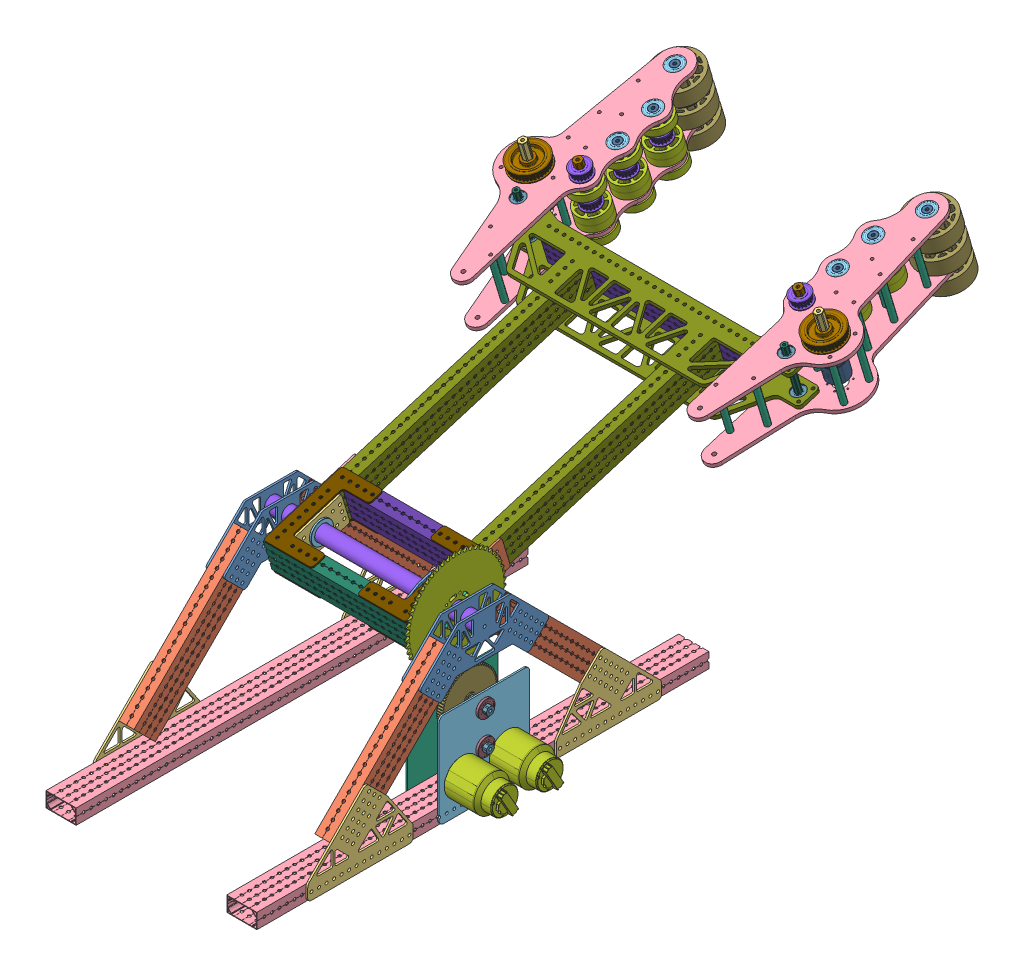
SolidWorks assembly Claw Assembly, configuration Default. Lengths in mm.
Overall size (590.37 576.41 1182.94).
222 component instances, 53 part files, 14 mates.
Components (placement in the parent):
- Side Assem 1-1: Side Assem 1 [Default] at (355.6 100.2071 0) size (53.97 279.4 762)
  - Top Gussest-1: Top Gussest [Default] at (-355.6 -95.25 -762) x (-1 0 0) z (0 0 -1) size (3.17 99.23 215.52)
  - Top Gussest-2: Top Gussest [Default] at (-330.2 -95.25 0) size (3.17 99.23 215.52)
  - 10.75in-1: 10.75in [Default] at (-342.9 31.4309 -149.9019) x (-1 0 0) z (0 -0.707107 0.707107) size (25.4 50.8 273.05)
  - 10.75in-2: 10.75in [Default] at (-342.9 31.4309 -612.0981) x (-1 0 0) z (0 -0.707107 -0.707107) size (25.4 50.8 273.05)
  - Bottom Gussest-1: Bottom Gussest [Default] at (-358.775 -95.25 0) size (3.17 121.55 177.8)
  - Bottom Gussest-2: Bottom Gussest [Default] at (-355.6 -95.25 -762) x (-1 0 0) z (0 0 -1) size (3.17 121.55 177.8)
  - 30in-1: 30in [Default] at (-330.2 -12.7 -12.7) x (0 -1 0) z (0 0 1) size (25.4 50.8 762)
- Side Assem 2-1: Side Assem 2 [Default] at (645.1703 93.5733 0) size (53.97 279.4 762)
  - Top Gussest-1: Top Gussest [Default] at (-289.5703 -88.6163 0) size (3.17 99.23 215.52)
  - Top Gussest-2: Top Gussest [Default] at (-314.9703 -88.6163 -762) x (-1 0 0) z (0 0 -1) size (3.17 99.23 215.52)
  - 10.75in-1: 10.75in [Default] at (-302.2703 38.0646 -612.0981) x (1 0 0) z (0 -0.707107 -0.707107) size (25.4 50.8 273.05)
  - 10.75in-2: 10.75in [Default] at (-302.2703 38.0646 -149.9019) x (1 0 0) z (0 -0.707107 0.707107) size (25.4 50.8 273.05)
  - Bottom Gussest-1: Bottom Gussest [Default] at (-286.3953 -88.6163 -762) x (-1 0 0) z (0 0 -1) size (3.17 121.55 177.8)
  - Bottom Gussest-2: Bottom Gussest [Default] at (-289.5703 -88.6163 0) size (3.17 121.55 177.8)
  - 30in-1: 30in [Default] at (-314.9703 -6.0663 -12.7) x (0 -1 0) z (0 0 1) size (25.4 50.8 762)
- Gearbox-1: Gearbox [Default] at (404.2822 133.0727 -812.0785) x (0 0 1) z (-1 0 0) size (152.4 182.49 147.05) (flexible)
  - Gearbox Plate-1: Gearbox Plate [Default] at (431.0785 -32.8657 46.1422) size (152.4 158.75 2.54)
  - Gearbox Plate 2-1: Gearbox Plate 2 [Default] at (431.0785 -32.8657 102.0222) x (-1 0 0) z (0 0 -1) size (152.4 158.75 2.54)
  - Falcon500_217-6515-1: Falcon500_217-6515 [Default] at (392.9785 -4.1633 19.9422) x (-1 0 0) z (0 0 1) size (60 60 115.81)
  - Falcon500_217-6515-2: Falcon500_217-6515 [Default] at (469.1785 -4.1633 19.9422) x (-1 0 0) z (0 0 1) size (60 60 115.81)
  - 12T Steel Spur Gear (20 DP, Falcon Motor) (217-6919).step-1: 12T Steel Spur Gear (20 DP, Falcon Motor) (217-6919).step [Default] at (392.9785 -4.1633 59.6672) x (-0.630647 0.77607 0) z (0 0 1) size (17.78 17.78 19.05)
  - 12T Steel Spur Gear (20 DP, Falcon Motor) (217-6919).step-2: 12T Steel Spur Gear (20 DP, Falcon Motor) (217-6919).step [Default] at (469.1785 -4.1633 59.6672) x (0.9345 -0.355964 0) z (0 0 1) size (17.78 17.78 19.05)
  - 15t steel hub sprocket hex boreWCP-0762-1: 15t steel hub sprocket hex boreWCP-0762 [Default] at (431.0785 76.9893 94.7959) x (-0.863195 -0.50487 0) z (0 0 -1) size (50.3 50.51 10.68)
  - 16T-1: 16T [Default] at (431.0785 21.1093 75.5935) x (-0.322756 0.946482 0) z (0 0 1) size (22.59 22.59 12.65)
  - 60T-1: 60T [Default] at (431.0785 21.1093 58.1818) x (0.322756 -0.946482 0) z (0 0 1) size (78.68 78.68 12.65)
  - 72T-2: 72T [Default] at (431.0785 76.9893 75.3268) x (-0.005633 0.999984 0) z (0 0 1) size (93.93 93.93 12.65)
  - Bearing-1: Bearing [Default] at (431.0785 21.1093 46.3009) x (0.706738 0.707475 0) z (0 0 1) size (31.12 31.12 7.94)
  - Bearing-3: Bearing [Default] at (431.0785 76.9893 101.8634) x (-0.628259 -0.778004 0) z (0 0 -1) size (31.12 31.12 7.94)
  - Bearing-4: Bearing [Default] at (431.0785 21.1093 101.8634) x (1 0 0) z (0 0 -1) size (31.12 31.12 7.94)
  - Bearing-5: Bearing [Default] at (431.0785 76.9893 46.3009) x (0.923728 0.383049 0) z (0 0 1) size (31.12 31.12 7.94)
  - Hex Stock-1: Hex Stock [Default] at (431.0785 21.1093 493.1822) x (0.752756 -0.658299 0) z (0 0 1) size (13.74 12.75 76.2)
  - Hex Stock-2: Hex Stock [Default] at (431.0785 76.9893 493.1822) x (-0.999984 -0.005633 0) z (0 0 1) size (13.74 12.75 76.2)
- Arm-1: Arm [Default] at (53.34 286.0719 -327.6042) x (1 0 0) z (0 -0.29021 0.956963) size (355.6 231.1 598.11) (flexible)
  - arm_tube_cross_back 9.5in-1: arm_tube_cross_back 9.5in [Default] at (228.6 25.4 -12.7) x (0 0 -1) z (1 0 0) size (25.4 50.8 241.3)
  - arm_tube 20.5in-1: arm_tube 20.5in [Default] at (228.6 25.4 -533.4) x (1 0 0) z (0 0 -1) size (25.4 50.8 520.7)
  - arm_tube 20.5in-2: arm_tube 20.5in [Default] at (12.7 25.4 -533.4) x (1 0 0) z (0 0 -1) size (25.4 50.8 520.7)
  - arm_tube_cross_front 7.5in-1: arm_tube_cross_front 7.5in [Default] at (38.1 25.4 -127) x (0 0 1) z (-1 0 0) size (25.4 50.8 190.5)
  - arm_body_bracket-1: arm_body_bracket [Default] at (-57.15 50.8 -457.2) x (0 0 1) z (0 1 0) size (139.7 82.55 2.54)
  - arm_body_bracket-2: arm_body_bracket [Default] at (298.45 53.34 -457.2) x (0 0 1) z (0 -1 0) size (139.7 82.55 2.54)
  - arm_pivot_mount_short-1: arm_pivot_mount_short [Default] at (212.725 25.4 -533.4) x (0 0 -1) z (1 0 0) size (82.55 63.5 3.17)
  - arm_pivot_mount-1: arm_pivot_mount [Default] at (241.3 25.4 -533.4) x (0 0 -1) z (1 0 0) size (139.7 63.5 3.17)
  - arm_pivot_short-1: arm_pivot_short [Default] at (25.4 25.4 -533.4) x (0 0 -1) z (1 0 0) size (82.55 50.8 3.17)
  - arm_pivot-1: arm_pivot [Default] at (-3.175 25.4 -533.4) x (0 0 -1) z (1 0 0) size (139.7 50.8 3.17)
  - 6338K436_Oil-Embedded Flanged Sleeve Bearing-2: 6338K436_Oil-Embedded Flanged Sleeve Bearing [6338K436] at (3.175 25.4 -63.5) x (0 -0.410084 -0.912048) z (-1 0 0) size (38.1 38.1 19.05)
  - 6338K436_Oil-Embedded Flanged Sleeve Bearing-3: 6338K436_Oil-Embedded Flanged Sleeve Bearing [6338K436] at (22.225 25.4 -63.5) x (0 -0.686347 0.727274) z (1 0 0) size (38.1 38.1 19.05)
  - 6338K436_Oil-Embedded Flanged Sleeve Bearing-4: 6338K436_Oil-Embedded Flanged Sleeve Bearing [6338K436] at (219.075 25.4 -63.5) x (0 -0.517801 -0.855501) z (-1 0 0) size (38.1 38.1 19.05)
  - 6338K436_Oil-Embedded Flanged Sleeve Bearing-5: 6338K436_Oil-Embedded Flanged Sleeve Bearing [6338K436] at (238.125 25.4 -63.5) x (0 -0.686347 0.727274) z (1 0 0) size (38.1 38.1 19.05)
  - arm_body_bracket-3: arm_body_bracket [Default] at (-57.15 -2.54 -457.2) x (0 0 1) z (0 1 0) size (139.7 82.55 2.54)
  - arm_body_bracket-4: arm_body_bracket [Default] at (298.45 0 -457.2) x (0 0 1) z (0 -1 0) size (139.7 82.55 2.54)
  - 3_8in spacer WCP-0309-1: 3_8in spacer WCP-0309 [Default] at (249.2375 46.0222 -75.4063) x (1 0 0) z (0 0.686347 -0.727274) size (9.53 9.5 9.5)
  - 54t #35 chain plate sprocket 217_2645-1: 54t #35 chain plate sprocket 217_2645 [Default] at (256.1463 25.4 -63.5) x (0 0.5 -0.866025) z (1 0 0) size (169.04 169.25 4.3)
  - 3_8in spacer WCP-0309-2: 3_8in spacer WCP-0309 [Default] at (249.2375 4.7778 -51.5938) x (1 0 0) z (0 0.686347 -0.727274) size (9.53 9.5 9.5)
  - 3_8in spacer WCP-0309-3: 3_8in spacer WCP-0309 [Default] at (249.2375 4.7778 -75.4063) x (1 0 0) z (0 0.686347 -0.727274) size (9.53 9.5 9.5)
  - 3_8in spacer WCP-0309-4: 3_8in spacer WCP-0309 [Default] at (249.2375 25.4 -39.6875) x (1 0 0) z (0 0.686347 -0.727274) size (9.53 9.5 9.5)
  - 3_8in spacer WCP-0309-5: 3_8in spacer WCP-0309 [Default] at (249.2375 46.0222 -51.5938) x (1 0 0) z (0 0.686347 -0.727274) size (9.53 9.5 9.5)
  - 3_8in spacer WCP-0309-6: 3_8in spacer WCP-0309 [Default] at (249.2375 25.4 -87.3125) x (1 0 0) z (0 0.686347 -0.727274) size (9.53 9.5 9.5)
  - tubemount-1: tubemount [Default] at (-53.34 25.4 -63.5) x (0 0.686347 -0.727274) z (-1 0 0) size (25.4 25.4 355.6)
- Roller Claw-1: Roller Claw [Default] at (-95.9547 241.4869 -1673.2272) x (1 0 0) z (0 -0.29021 0.956963) size (590.37 159.05 455.23)
  - Right Roller Claw-1: Right Roller Claw [Default] at (339.7553 150.3563 318.0728) size (145.49 159.05 454.48)
    - 36T_HTD_5mmP_9mmW_flanged_500_hex_217-3231-1: 36T_HTD_5mmP_9mmW_flanged_500_hex_217-3231 [Default] at (179.6545 359.9234 345.8295) x (-0.337159 0 -0.941448) z (0 -1 0) size (60 60 14.5)
    - ultraplanetary-1: ultraplanetary [Default] at (198.2743 320.0734 349.6112) x (-0.199034 0 0.979992) z (0 -1 0) size (63.81 63.81 121.86)
      - REV-21-1651-1: REV-21-1651 [Default] at (0 19 -11.5) x (0 0 1) z (-0.999972 -0.007497 0) size (56.01 42.91 43.01)
      - REV-41-1601-1: REV-41-1601 [Default] at (0 19 -10) x (-0.5 -0.866025 0) z (0 0 1) size (43.62 38.42 17.88)
      - REV-41-1604-1: REV-41-1604 [Default] at (0 19 -26.25) x (-0.5 0.866025 0) z (0 0 1) size (54.69 56.73 18.25)
        - REV-41-1604.STEP-1: REV-41-1604.STEP [Default] at origin size (54.69 56.73 18.25)
          - REV-41-1604-2.STEP-1: REV-41-1604-2.STEP [Default] at origin size (43.57 38 6.25)
          - REV-41-1604-1.STEP-1: REV-41-1604-1.STEP [Default] at (0 0 7) x (0.5 0.866025 0) z (0 0 -1) size (43.57 38 7.03)
          - 6704ZZ.STEP-1: 6704ZZ.STEP [Default] at (0 0 7.75) x (0.995 -0.099871 0) z (0 0 1) size (27 27 4)
          - 6704ZZ.STEP-2: 6704ZZ.STEP [Default] at (0 0 3) x (0.993119 0.117109 0) z (0 0 1) size (27 27 4)
          - REV-40-1606_Through Hole.STEP-1: REV-40-1606_Through Hole.STEP [Default] at (0 0 10.95) x (-0.517794 -0.855505 0) z (0 0 -1) size (22 22 16.95)
          - REV-41-1604-4.STEP-1: REV-41-1604-4.STEP [Default] at (0 0 9.7) x (0.517794 0.855505 0) z (0 0 1) size (22 22 1.25)
          - REV-41-1604-3.STEP-1: REV-41-1604-3.STEP [Default] at (0 0 5) size (27.02 27 1.12)
          - socket head cap screw_am_B18.3.1M - 2 x 0.4 x 4 Hex SHCS -- 4NHX.STEP-1: socket head cap screw_am_B18.3.1M - 2 x 0.4 x 4 Hex SHCS -- 4NHX.STEP [Default] at (-11.8435 -10.7579 11.2) x (0 0 -1) z (-0.492915 -0.870077 0) size (6 3.8 3.8)
          - socket head cap screw_am_B18.3.1M - 2 x 0.4 x 4 Hex SHCS -- 4NHX.STEP-2: socket head cap screw_am_B18.3.1M - 2 x 0.4 x 4 Hex SHCS -- 4NHX.STEP [Default] at (-3.3948 15.6357 11.2) x (0 0 -1) z (-0.934724 -0.355374 0) size (6 3.8 3.8)
          - socket head cap screw_am_B18.3.1M - 2 x 0.4 x 4 Hex SHCS -- 4NHX.STEP-3: socket head cap screw_am_B18.3.1M - 2 x 0.4 x 4 Hex SHCS -- 4NHX.STEP [Default] at (15.2383 -4.8778 11.2) x (0 0 -1) z (0.970727 -0.240185 0) size (6 3.8 3.8)
          - 91294A003_BLACK ALLOY STEEL FLAT-HEAD SOCKET CAP SCREW_91294A003.STEP-1: 91294A003_BLACK ALLOY STEEL FLAT-HEAD SOCKET CAP SCREW_91294A003.STEP [Default] at (6.5084 3.5803 10.95) size (4 4 5)
          - 91294A003_BLACK ALLOY STEEL FLAT-HEAD SOCKET CAP SCREW_91294A003.STEP-2: 91294A003_BLACK ALLOY STEEL FLAT-HEAD SOCKET CAP SCREW_91294A003.STEP [Default] at (-0.1535 -7.4266 10.95) size (4 4 5)
          - 91294A003_BLACK ALLOY STEEL FLAT-HEAD SOCKET CAP SCREW_91294A003.STEP-3: 91294A003_BLACK ALLOY STEEL FLAT-HEAD SOCKET CAP SCREW_91294A003.STEP [Default] at (-6.3549 3.8463 10.95) size (4 4 5)
      - REV-41-1607-1: REV-41-1607 [Default] at (0 19 0) x (-1 0 0) z (0 -1 0) size (43.57 5 38.01)
      - REV-41-1620-1: REV-41-1620 [Default] at (0 19 -32.25) x (0.876175 0.481992 0) z (0 0 1) size (22 22 46.85)
    - Claw Plates-2: Claw Plates [Default] at (-69.8106 346.3234 416.9495) size (132.77 6.35 429.09)
    - thunderhex_flanged_217-4006-10: thunderhex_flanged_217-4006 [Default] at (115.7867 348.7046 321.0569) x (0.592492 0 0.805576) z (0 -1 0) size (31.12 31.12 7.94)
    - thunderhex_flanged_217-4006-11: thunderhex_flanged_217-4006 [Default] at (115.7867 348.7046 258.5475) x (-0.906539 0 -0.422123) z (0 -1 0) size (31.12 31.12 7.94)
    - thunderhex_flanged_217-4006-12: thunderhex_flanged_217-4006 [Default] at (115.7867 348.7046 196.0381) x (-0.994435 0 -0.105355) z (0 -1 0) size (31.12 31.12 7.94)
    - thunderhex_flanged_217-4006-13: thunderhex_flanged_217-4006 [Default] at (142.9222 348.7046 129.5022) x (0.097157 0 0.995269) z (0 -1 0) size (31.12 31.12 7.94)
    - Claw Plates-1: Claw Plates [Default] at (-69.8106 263.7734 416.9495) size (132.77 6.35 429.09)
    - thunderhex_flanged_217-4006-1: thunderhex_flanged_217-4006 [Default] at (115.7867 267.7421 321.0569) x (0.900767 0 -0.434303) z (0 1 0) size (31.12 31.12 7.94)
    - thunderhex_flanged_217-4006-3: thunderhex_flanged_217-4006 [Default] at (115.7867 267.7421 258.5475) x (-0.989804 0 -0.142438) z (0 1 0) size (31.12 31.12 7.94)
    - thunderhex_flanged_217-4006-4: thunderhex_flanged_217-4006 [Default] at (115.7867 267.7421 196.0381) x (-0.890133 0 -0.4557) z (0 1 0) size (31.12 31.12 7.94)
    - thunderhex_flanged_217-4006-5: thunderhex_flanged_217-4006 [Default] at (142.9222 267.7421 129.5022) x (-0.890133 0 -0.4557) z (0 1 0) size (31.12 31.12 7.94)
    - 3_000_L_10_thru_WCP-0209-1: 3_000_L_10_thru_WCP-0209 [Default] at (120.1277 308.2234 477.6333) x (0 1 0) z (-0.241352 0 0.970438) size (76.2 9.5 9.5)
    - 3_000_L_10_thru_WCP-0209-2: 3_000_L_10_thru_WCP-0209 [Default] at (151.8777 308.2234 444.6133) x (0 1 0) z (-0.241352 0 0.970438) size (76.2 9.5 9.5)
    - 3_000_L_10_thru_WCP-0209-3: 3_000_L_10_thru_WCP-0209 [Default] at (141.5239 308.2234 345.4022) x (0 1 0) z (-0.241352 0 0.970438) size (76.2 9.5 9.5)
    - 3_000_L_10_thru_WCP-0209-4: 3_000_L_10_thru_WCP-0209 [Default] at (207.4135 308.2234 368.0545) x (0 1 0) z (-0.241352 0 0.970438) size (76.2 9.5 9.5)
    - 3_000_L_10_thru_WCP-0209-5: 3_000_L_10_thru_WCP-0209 [Default] at (207.4135 308.2234 323.6045) x (0 -1 0) z (-0.328723 0 0.944426) size (76.2 9.5 9.5)
    - 3_000_L_10_thru_WCP-0209-6: 3_000_L_10_thru_WCP-0209 [Default] at (170.8852 308.2234 287.9041) x (0 1 0) z (-0.241352 0 0.970438) size (76.2 9.5 9.5)
    - 3_000_L_10_thru_WCP-0209-7: 3_000_L_10_thru_WCP-0209 [Default] at (141.5239 308.2234 288.2522) x (0 1 0) z (-0.241352 0 0.970438) size (76.2 9.5 9.5)
    - 3_000_L_10_thru_WCP-0209-8: 3_000_L_10_thru_WCP-0209 [Default] at (166.9239 308.2234 237.2588) x (0 1 0) z (-0.241352 0 0.970438) size (76.2 9.5 9.5)
    - 3_000_L_10_thru_WCP-0209-9: 3_000_L_10_thru_WCP-0209 [Default] at (141.5239 308.2234 224.7522) x (0 1 0) z (-0.241352 0 0.970438) size (76.2 9.5 9.5)
    - 3_000_L_10_thru_WCP-0209-10: 3_000_L_10_thru_WCP-0209 [Default] at (161.9722 308.2234 173.9522) x (0 1 0) z (-0.241352 0 0.970438) size (76.2 9.5 9.5)
    - 2_OD_30A_Straight_Flex_Wheel_217-6353-1: 2_OD_30A_Straight_Flex_Wheel_217-6353 [Default] at (115.7867 293.7234 321.0569) x (-0.99292 0 0.118786) z (0.118786 0 0.99292) size (50.8 12.7 50.8)
    - 18T_HTD_5mmP_9mmW_flanged_500_hex_217-3225-2: 18T_HTD_5mmP_9mmW_flanged_500_hex_217-3225 [Default] at (115.7867 307.3234 321.0569) x (-0.800501 0 0.599331) z (0 -1 0) size (32 32 14.5)
    - 18T_HTD_5mmP_9mmW_flanged_500_hex_217-3225-1: 18T_HTD_5mmP_9mmW_flanged_500_hex_217-3225 [Default] at (115.7867 321.8234 321.0569) x (-0.800501 0 0.599331) z (0 1 0) size (32 32 14.5)
    - 2_OD_30A_Straight_Flex_Wheel_217-6353-3: 2_OD_30A_Straight_Flex_Wheel_217-6353 [Default] at (115.7867 335.4234 321.0569) x (-0.99292 0 0.118786) z (0.118786 0 0.99292) size (50.8 12.7 50.8)
    - 2_OD_30A_Straight_Flex_Wheel_217-6353-2: 2_OD_30A_Straight_Flex_Wheel_217-6353 [Default] at (115.7867 281.0234 321.0569) x (-0.99292 0 0.118786) z (0.118786 0 0.99292) size (50.8 12.7 50.8)
    - 2_OD_30A_Straight_Flex_Wheel_217-6353-13: 2_OD_30A_Straight_Flex_Wheel_217-6353 [Default] at (115.7867 257.4234 321.0569) x (-0.99292 0 0.118786) z (0.118786 0 0.99292) size (50.8 12.7 50.8)
    - 1_2thunderhex_5.5in-1: 1_2thunderhex_5.5in [Default] at (115.7867 695.5734 321.0569) x (-0.919287 0 -0.393589) z (0 -1 0) size (13.74 12.75 139.7)
    - 18T_HTD_5mmP_9mmW_flanged_500_hex_217-3225-9: 18T_HTD_5mmP_9mmW_flanged_500_hex_217-3225 [Default] at (115.7867 359.9234 321.0569) x (-0.800501 0 0.599331) z (0 -1 0) size (32 32 14.5)
    - 2_OD_30A_Straight_Flex_Wheel_217-6353-7: 2_OD_30A_Straight_Flex_Wheel_217-6353 [Default] at (115.7867 293.7234 258.5475) x (-0.956763 0 0.290869) z (0.290869 0 0.956763) size (50.8 12.7 50.8)
    - 18T_HTD_5mmP_9mmW_flanged_500_hex_217-3225-5: 18T_HTD_5mmP_9mmW_flanged_500_hex_217-3225 [Default] at (115.7867 307.3234 258.5475) x (-0.683146 0 0.730282) z (0 -1 0) size (32 32 14.5)
    - 18T_HTD_5mmP_9mmW_flanged_500_hex_217-3225-6: 18T_HTD_5mmP_9mmW_flanged_500_hex_217-3225 [Default] at (115.7867 321.8234 258.5475) x (-0.683146 0 0.730282) z (0 1 0) size (32 32 14.5)
    - 2_OD_30A_Straight_Flex_Wheel_217-6353-8: 2_OD_30A_Straight_Flex_Wheel_217-6353 [Default] at (115.7867 335.4234 258.5475) x (-0.956763 0 0.290869) z (0.290869 0 0.956763) size (50.8 12.7 50.8)
    - 2_OD_30A_Straight_Flex_Wheel_217-6353-9: 2_OD_30A_Straight_Flex_Wheel_217-6353 [Default] at (115.7867 281.0234 258.5475) x (-0.956763 0 0.290869) z (0.290869 0 0.956763) size (50.8 12.7 50.8)
    - 1_2thunderhex_4.5in-2: 1_2thunderhex_4.5in [Default] at (115.7867 695.5734 258.5475) x (0.683146 0 -0.730282) z (0 -1 0) size (13.74 12.75 114.3)
    - 2_OD_30A_Straight_Flex_Wheel_217-6353-14: 2_OD_30A_Straight_Flex_Wheel_217-6353 [Default] at (115.7867 257.4234 258.5475) x (-0.730282 0 -0.683146) z (-0.683146 0 0.730282) size (50.8 12.7 50.8)
    - 2_OD_30A_Straight_Flex_Wheel_217-6353-10: 2_OD_30A_Straight_Flex_Wheel_217-6353 [Default] at (115.7867 293.7234 196.0381) x (0.94551 0 -0.325593) z (-0.325593 0 -0.94551) size (50.8 12.7 50.8)
    - 18T_HTD_5mmP_9mmW_flanged_500_hex_217-3225-7: 18T_HTD_5mmP_9mmW_flanged_500_hex_217-3225 [Default] at (115.7867 307.3234 196.0381) x (0.656039 0 -0.754727) z (0 -1 0) size (32 32 14.5)
    - 18T_HTD_5mmP_9mmW_flanged_500_hex_217-3225-8: 18T_HTD_5mmP_9mmW_flanged_500_hex_217-3225 [Default] at (115.7867 321.8234 196.0381) x (0.656039 0 -0.754727) z (0 1 0) size (32 32 14.5)
    - 2_OD_30A_Straight_Flex_Wheel_217-6353-11: 2_OD_30A_Straight_Flex_Wheel_217-6353 [Default] at (115.7867 335.4234 196.0381) x (0.94551 0 -0.325593) z (-0.325593 0 -0.94551) size (50.8 12.7 50.8)
    - 2_OD_30A_Straight_Flex_Wheel_217-6353-12: 2_OD_30A_Straight_Flex_Wheel_217-6353 [Default] at (115.7867 281.0234 196.0381) x (0.94551 0 -0.325593) z (-0.325593 0 -0.94551) size (50.8 12.7 50.8)
    - 1_2thunderhex_4.5in-3: 1_2thunderhex_4.5in [Default] at (115.7867 695.5734 196.0381) x (0.656039 0 -0.754727) z (0 -1 0) size (13.74 12.75 114.3)
    - 2_OD_30A_Straight_Flex_Wheel_217-6353-15: 2_OD_30A_Straight_Flex_Wheel_217-6353 [Default] at (115.7867 257.4234 196.0381) x (-0.190783 0 0.981632) z (0.981632 0 0.190783) size (50.8 12.7 50.8)
    - wide_roller_wheel-1: wide_roller_wheel [Default] at (123.4101 254.2514 114.098) x (-0.521403 0 0.853311) z (-0.853311 0 -0.521403) size (76.2 25.4 76.2)
      - wide_wheel_mount-1: wide_wheel_mount [Default] at (2.9708 21.322 -24.6817) size (28.57 25.4 28.57)
      - 3_OD_30A_Straight_Flex_Wheel-1: 3_OD_30A_Straight_Flex_Wheel [Default] at (2.9708 34.022 -24.6817) size (76.2 25.4 76.2)
    - wide_roller_wheel-2: wide_roller_wheel [Default] at (123.4101 294.1514 114.098) x (-0.521403 0 0.853311) z (-0.853311 0 -0.521403) size (76.2 25.4 76.2)
      - wide_wheel_mount-1: wide_wheel_mount [Default] at (2.9708 21.322 -24.6817) size (28.57 25.4 28.57)
      - 3_OD_30A_Straight_Flex_Wheel-1: 3_OD_30A_Straight_Flex_Wheel [Default] at (2.9708 34.022 -24.6817) size (76.2 25.4 76.2)
    - 30T_HTD_5mmP_9mmW_flanged_500_hex_217-3229-2: 30T_HTD_5mmP_9mmW_flanged_500_hex_217-3229 [Default] at (142.9222 308.2234 129.5022) x (0.521403 0 -0.853311) z (0 1 0) size (51 51 14.5)
    - 1_2thunderhex_4.5in-4: 1_2thunderhex_4.5in [Default] at (142.9222 695.5734 129.5022) x (-0.99969 0 -0.024892) z (0 -1 0) size (13.74 12.75 114.3)
    - wide_roller_wheel-3: wide_roller_wheel [Default] at (162.4344 217.0514 144.9063) x (0.521403 0 -0.853311) z (0.853311 0 0.521403) size (76.2 25.4 76.2)
      - wide_wheel_mount-1: wide_wheel_mount [Default] at (2.9708 21.322 -24.6817) size (28.57 25.4 28.57)
      - 3_OD_30A_Straight_Flex_Wheel-1: 3_OD_30A_Straight_Flex_Wheel [Default] at (2.9708 34.022 -24.6817) size (76.2 25.4 76.2)
    - thunderhex_375_flanged_217-5829-1: thunderhex_375_flanged_217-5829 [Default] at (156.2494 344.7359 391.5495) x (0 1 0) z (-0.397184 0 0.917739) size (7.11 24.61 24.61)
    - thunderhex_375_flanged_217-5829-2: thunderhex_375_flanged_217-5829 [Default] at (156.2494 271.7109 391.5495) x (0 -1 0) z (0 0 1) size (7.11 24.61 24.61)
    - 3_8thunderhex_4.5in-1: 3_8thunderhex_4.5in [Default] at (156.2494 -91.8266 391.5495) x (0.142102 0 -0.989852) z (0 -1 0) size (10.24 9.53 114.3)
    - thunderhex_375_flanged_217-5829-3: thunderhex_375_flanged_217-5829 [Default] at (156.2494 274.8859 391.5495) x (0 1 0) z (0.329672 0 -0.944096) size (7.11 24.61 24.61)
    - thunderhex_375_flanged_217-5829-4: thunderhex_375_flanged_217-5829 [Default] at (156.2494 341.5609 391.5495) x (0 -1 0) z (0.640533 0 0.76793) size (7.11 24.61 24.61)
  - Left Roller Claw-1: Left Roller Claw [Default] at (-161.3847 238.4838 416.2723) size (145.24 159.05 455.23)
    - 36T_HTD_5mmP_9mmW_flanged_500_hex_217-3231-1: 36T_HTD_5mmP_9mmW_flanged_500_hex_217-3231 [Default] at (181.8644 271.7959 247.63) x (0.29796 0 -0.954578) z (0 -1 0) size (60 60 14.5)
    - ultraplanetary-1: ultraplanetary [Default] at (194.4494 231.9459 261.8645) x (-0.749181 0 0.662365) z (0 -1 0) size (63.81 63.81 121.86)
      - REV-21-1651-1: REV-21-1651 [Default] at (0 19 -11.5) x (0 0 1) z (-0.999972 -0.007497 0) size (56.01 42.91 43.01)
      - REV-41-1601-1: REV-41-1601 [Default] at (0 19 -10) x (-0.5 -0.866025 0) z (0 0 1) size (43.62 38.42 17.88)
      - REV-41-1604-1: REV-41-1604 [Default] at (0 19 -26.25) x (-0.5 0.866025 0) z (0 0 1) size (54.69 56.73 18.25)
        - REV-41-1604.STEP-1: REV-41-1604.STEP [Default] at origin size (54.69 56.73 18.25)
          - REV-41-1604-2.STEP-1: REV-41-1604-2.STEP [Default] at origin size (43.57 38 6.25)
          - REV-41-1604-1.STEP-1: REV-41-1604-1.STEP [Default] at (0 0 7) x (0.5 0.866025 0) z (0 0 -1) size (43.57 38 7.03)
          - 6704ZZ.STEP-1: 6704ZZ.STEP [Default] at (0 0 7.75) x (0.995 -0.099871 0) z (0 0 1) size (27 27 4)
          - 6704ZZ.STEP-2: 6704ZZ.STEP [Default] at (0 0 3) x (0.993119 0.117109 0) z (0 0 1) size (27 27 4)
          - REV-40-1606_Through Hole.STEP-1: REV-40-1606_Through Hole.STEP [Default] at (0 0 10.95) x (-0.517794 -0.855505 0) z (0 0 -1) size (22 22 16.95)
          - REV-41-1604-4.STEP-1: REV-41-1604-4.STEP [Default] at (0 0 9.7) x (0.517794 0.855505 0) z (0 0 1) size (22 22 1.25)
          - REV-41-1604-3.STEP-1: REV-41-1604-3.STEP [Default] at (0 0 5) size (27.02 27 1.12)
          - socket head cap screw_am_B18.3.1M - 2 x 0.4 x 4 Hex SHCS -- 4NHX.STEP-1: socket head cap screw_am_B18.3.1M - 2 x 0.4 x 4 Hex SHCS -- 4NHX.STEP [Default] at (-11.8435 -10.7579 11.2) x (0 0 -1) z (-0.492915 -0.870077 0) size (6 3.8 3.8)
          - socket head cap screw_am_B18.3.1M - 2 x 0.4 x 4 Hex SHCS -- 4NHX.STEP-2: socket head cap screw_am_B18.3.1M - 2 x 0.4 x 4 Hex SHCS -- 4NHX.STEP [Default] at (-3.3948 15.6357 11.2) x (0 0 -1) z (-0.934724 -0.355374 0) size (6 3.8 3.8)
          - socket head cap screw_am_B18.3.1M - 2 x 0.4 x 4 Hex SHCS -- 4NHX.STEP-3: socket head cap screw_am_B18.3.1M - 2 x 0.4 x 4 Hex SHCS -- 4NHX.STEP [Default] at (15.2383 -4.8778 11.2) x (0 0 -1) z (0.970727 -0.240185 0) size (6 3.8 3.8)
          - 91294A003_BLACK ALLOY STEEL FLAT-HEAD SOCKET CAP SCREW_91294A003.STEP-1: 91294A003_BLACK ALLOY STEEL FLAT-HEAD SOCKET CAP SCREW_91294A003.STEP [Default] at (6.5084 3.5803 10.95) size (4 4 5)
          - 91294A003_BLACK ALLOY STEEL FLAT-HEAD SOCKET CAP SCREW_91294A003.STEP-2: 91294A003_BLACK ALLOY STEEL FLAT-HEAD SOCKET CAP SCREW_91294A003.STEP [Default] at (-0.1535 -7.4266 10.95) size (4 4 5)
          - 91294A003_BLACK ALLOY STEEL FLAT-HEAD SOCKET CAP SCREW_91294A003.STEP-3: 91294A003_BLACK ALLOY STEEL FLAT-HEAD SOCKET CAP SCREW_91294A003.STEP [Default] at (-6.3549 3.8463 10.95) size (4 4 5)
      - REV-41-1607-1: REV-41-1607 [Default] at (0 19 0) x (-1 0 0) z (0 -1 0) size (43.57 5 38.01)
      - REV-41-1620-1: REV-41-1620 [Default] at (0 19 -32.25) x (0.876175 0.481992 0) z (0 0 1) size (22 22 46.85)
    - Claw Plates-2: Claw Plates [Default] at (431.3295 264.5459 318.75) x (-1 0 0) z (0 0 1) size (132.77 6.35 429.09)
    - thunderhex_flanged_217-4006-10: thunderhex_flanged_217-4006 [Default] at (245.7322 260.5771 222.8574) x (0.592492 0 0.805576) z (0 -1 0) size (31.12 31.12 7.94)
    - thunderhex_flanged_217-4006-11: thunderhex_flanged_217-4006 [Default] at (245.7322 260.5771 160.348) x (-0.906539 0 -0.422123) z (0 -1 0) size (31.12 31.12 7.94)
    - thunderhex_flanged_217-4006-12: thunderhex_flanged_217-4006 [Default] at (245.7322 260.5771 97.8386) x (-0.881857 0 -0.471518) z (0 -1 0) size (31.12 31.12 7.94)
    - thunderhex_flanged_217-4006-13: thunderhex_flanged_217-4006 [Default] at (218.5967 260.5771 31.3027) x (0.097157 0 0.995269) z (0 -1 0) size (31.12 31.12 7.94)
    - Claw Plates-1: Claw Plates [Default] at (431.3295 181.9959 318.75) x (-1 0 0) z (0 0 1) size (132.77 6.35 429.09)
    - thunderhex_flanged_217-4006-1: thunderhex_flanged_217-4006 [Default] at (245.7322 179.6146 222.8574) x (0.900767 0 -0.434303) z (0 1 0) size (31.12 31.12 7.94)
    - thunderhex_flanged_217-4006-3: thunderhex_flanged_217-4006 [Default] at (245.7322 179.6146 160.348) x (-0.989504 0 -0.144504) z (0 1 0) size (31.12 31.12 7.94)
    - thunderhex_flanged_217-4006-4: thunderhex_flanged_217-4006 [Default] at (245.7322 179.6146 97.8386) x (-0.243579 0 -0.969881) z (0 1 0) size (31.12 31.12 7.94)
    - thunderhex_flanged_217-4006-5: thunderhex_flanged_217-4006 [Default] at (218.5967 179.6146 31.3027) x (-0.890339 0 -0.455299) z (0 1 0) size (31.12 31.12 7.94)
    - 3_000_L_10_thru_WCP-0209-1: 3_000_L_10_thru_WCP-0209 [Default] at (219.995 220.0959 247.2027) x (0 1 0) z (-0.241352 0 0.970438) size (76.2 9.5 9.5)
    - 3_000_L_10_thru_WCP-0209-2: 3_000_L_10_thru_WCP-0209 [Default] at (241.3912 220.0959 379.4338) x (0 1 0) z (-0.241352 0 0.970438) size (76.2 9.5 9.5)
    - 3_000_L_10_thru_WCP-0209-3: 3_000_L_10_thru_WCP-0209 [Default] at (154.1054 220.0959 225.405) x (0 1 0) z (-0.241352 0 0.970438) size (76.2 9.5 9.5)
    - 3_000_L_10_thru_WCP-0209-4: 3_000_L_10_thru_WCP-0209 [Default] at (209.6412 220.0959 346.4138) x (0 1 0) z (-0.241352 0 0.970438) size (76.2 9.5 9.5)
    - 3_000_L_10_thru_WCP-0209-5: 3_000_L_10_thru_WCP-0209 [Default] at (154.1054 220.0959 269.855) x (0 -1 0) z (-0.328723 0 0.944426) size (76.2 9.5 9.5)
    - 3_000_L_10_thru_WCP-0209-6: 3_000_L_10_thru_WCP-0209 [Default] at (190.6337 220.0959 189.7046) x (0 1 0) z (-0.241352 0 0.970438) size (76.2 9.5 9.5)
    - 3_000_L_10_thru_WCP-0209-7: 3_000_L_10_thru_WCP-0209 [Default] at (219.995 220.0959 190.0527) x (0 1 0) z (-0.241352 0 0.970438) size (76.2 9.5 9.5)
    - 3_000_L_10_thru_WCP-0209-8: 3_000_L_10_thru_WCP-0209 [Default] at (194.595 220.0959 139.0593) x (0 1 0) z (-0.241352 0 0.970438) size (76.2 9.5 9.5)
    - 3_000_L_10_thru_WCP-0209-9: 3_000_L_10_thru_WCP-0209 [Default] at (219.995 220.0959 126.5527) x (0 1 0) z (-0.241352 0 0.970438) size (76.2 9.5 9.5)
    - 3_000_L_10_thru_WCP-0209-10: 3_000_L_10_thru_WCP-0209 [Default] at (199.5467 220.0959 75.7527) x (0 -1 0) z (0.241352 0 0.970438) size (76.2 9.5 9.5)
    - 2_OD_30A_Straight_Flex_Wheel_217-6353-1: 2_OD_30A_Straight_Flex_Wheel_217-6353 [Default] at (245.7322 205.5959 222.8574) x (0.111174 0 -0.993801) z (-0.993801 0 -0.111174) size (50.8 12.7 50.8)
    - 18T_HTD_5mmP_9mmW_flanged_500_hex_217-3225-2: 18T_HTD_5mmP_9mmW_flanged_500_hex_217-3225 [Default] at (245.7322 219.1959 222.8574) x (-0.400621 0 -0.916244) z (0 -1 0) size (32 32 14.5)
    - 18T_HTD_5mmP_9mmW_flanged_500_hex_217-3225-1: 18T_HTD_5mmP_9mmW_flanged_500_hex_217-3225 [Default] at (245.7322 233.6959 222.8574) x (-0.400621 0 -0.916244) z (0 1 0) size (32 32 14.5)
    - 2_OD_30A_Straight_Flex_Wheel_217-6353-3: 2_OD_30A_Straight_Flex_Wheel_217-6353 [Default] at (245.7322 247.2959 222.8574) x (0.111174 0 -0.993801) z (-0.993801 0 -0.111174) size (50.8 12.7 50.8)
    - 2_OD_30A_Straight_Flex_Wheel_217-6353-2: 2_OD_30A_Straight_Flex_Wheel_217-6353 [Default] at (245.7322 192.8959 222.8574) x (0.111174 0 -0.993801) z (-0.993801 0 -0.111174) size (50.8 12.7 50.8)
    - 2_OD_30A_Straight_Flex_Wheel_217-6353-13: 2_OD_30A_Straight_Flex_Wheel_217-6353 [Default] at (245.7322 169.2959 222.8574) x (0.111174 0 -0.993801) z (-0.993801 0 -0.111174) size (50.8 12.7 50.8)
    - 1_2thunderhex_5.5in-1: 1_2thunderhex_5.5in [Default] at (245.7322 607.4459 222.8574) x (0.59318 0 -0.80507) z (0 -1 0) size (13.74 12.75 139.7)
    - 18T_HTD_5mmP_9mmW_flanged_500_hex_217-3225-9: 18T_HTD_5mmP_9mmW_flanged_500_hex_217-3225 [Default] at (245.7322 271.7959 222.8574) x (-0.400621 0 -0.916244) z (0 -1 0) size (32 32 14.5)
    - 2_OD_30A_Straight_Flex_Wheel_217-6353-7: 2_OD_30A_Straight_Flex_Wheel_217-6353 [Default] at (245.7322 205.5959 160.348) x (0.996179 0 -0.087336) z (-0.087336 0 -0.996179) size (50.8 12.7 50.8)
    - 18T_HTD_5mmP_9mmW_flanged_500_hex_217-3225-5: 18T_HTD_5mmP_9mmW_flanged_500_hex_217-3225 [Default] at (245.7322 219.1959 160.348) x (0.819048 0 -0.573725) z (0 -1 0) size (32 32 14.5)
    - 18T_HTD_5mmP_9mmW_flanged_500_hex_217-3225-6: 18T_HTD_5mmP_9mmW_flanged_500_hex_217-3225 [Default] at (245.7322 233.6959 160.348) x (0.819048 0 -0.573725) z (0 1 0) size (32 32 14.5)
    - 2_OD_30A_Straight_Flex_Wheel_217-6353-8: 2_OD_30A_Straight_Flex_Wheel_217-6353 [Default] at (245.7322 247.2959 160.348) x (0.996179 0 -0.087336) z (-0.087336 0 -0.996179) size (50.8 12.7 50.8)
    - 2_OD_30A_Straight_Flex_Wheel_217-6353-9: 2_OD_30A_Straight_Flex_Wheel_217-6353 [Default] at (245.7322 192.8959 160.348) x (0.996179 0 -0.087336) z (-0.087336 0 -0.996179) size (50.8 12.7 50.8)
    - 1_2thunderhex_4.5in-2: 1_2thunderhex_4.5in [Default] at (245.7322 607.4459 160.348) x (-0.819048 0 0.573725) z (0 -1 0) size (13.74 12.75 114.3)
    - 2_OD_30A_Straight_Flex_Wheel_217-6353-14: 2_OD_30A_Straight_Flex_Wheel_217-6353 [Default] at (245.7322 169.2959 160.348) x (0.573725 0 0.819048) z (0.819048 0 -0.573725) size (50.8 12.7 50.8)
    - 2_OD_30A_Straight_Flex_Wheel_217-6353-10: 2_OD_30A_Straight_Flex_Wheel_217-6353 [Default] at (245.7322 205.5959 97.8386) x (0.37446 0 -0.927243) z (-0.927243 0 -0.37446) size (50.8 12.7 50.8)
    - 18T_HTD_5mmP_9mmW_flanged_500_hex_217-3225-7: 18T_HTD_5mmP_9mmW_flanged_500_hex_217-3225 [Default] at (245.7322 219.1959 97.8386) x (-0.139329 0 -0.990246) z (0 -1 0) size (32 32 14.5)
    - 18T_HTD_5mmP_9mmW_flanged_500_hex_217-3225-8: 18T_HTD_5mmP_9mmW_flanged_500_hex_217-3225 [Default] at (245.7322 233.6959 97.8386) x (-0.139329 0 -0.990246) z (0 1 0) size (32 32 14.5)
    - 2_OD_30A_Straight_Flex_Wheel_217-6353-11: 2_OD_30A_Straight_Flex_Wheel_217-6353 [Default] at (245.7322 247.2959 97.8386) x (0.37446 0 -0.927243) z (-0.927243 0 -0.37446) size (50.8 12.7 50.8)
    - 2_OD_30A_Straight_Flex_Wheel_217-6353-12: 2_OD_30A_Straight_Flex_Wheel_217-6353 [Default] at (245.7322 192.8959 97.8386) x (0.37446 0 -0.927243) z (-0.927243 0 -0.37446) size (50.8 12.7 50.8)
    - 1_2thunderhex_4.5in-3: 1_2thunderhex_4.5in [Default] at (245.7322 607.4459 97.8386) x (-0.139329 0 -0.990246) z (0 -1 0) size (13.74 12.75 114.3)
    - 2_OD_30A_Straight_Flex_Wheel_217-6353-15: 2_OD_30A_Straight_Flex_Wheel_217-6353 [Default] at (245.7322 169.2959 97.8386) x (0.615786 0 0.787914) z (0.787914 0 -0.615786) size (50.8 12.7 50.8)
    - wide_roller_wheel-1: wide_roller_wheel [Default] at (230.4702 166.1239 53.1437) x (0.815195 0 -0.579187) z (0.579187 0 0.815195) size (76.2 25.4 76.2)
      - wide_wheel_mount-1: wide_wheel_mount [Default] at (2.9708 21.322 -24.6817) size (28.57 25.4 28.57)
      - 3_OD_30A_Straight_Flex_Wheel-1: 3_OD_30A_Straight_Flex_Wheel [Default] at (2.9708 34.022 -24.6817) size (76.2 25.4 76.2)
    - wide_roller_wheel-2: wide_roller_wheel [Default] at (230.4702 206.0239 53.1437) x (0.815195 0 -0.579187) z (0.579187 0 0.815195) size (76.2 25.4 76.2)
      - wide_wheel_mount-1: wide_wheel_mount [Default] at (2.9708 21.322 -24.6817) size (28.57 25.4 28.57)
      - 3_OD_30A_Straight_Flex_Wheel-1: 3_OD_30A_Straight_Flex_Wheel [Default] at (2.9708 34.022 -24.6817) size (76.2 25.4 76.2)
    - 30T_HTD_5mmP_9mmW_flanged_500_hex_217-3229-2: 30T_HTD_5mmP_9mmW_flanged_500_hex_217-3229 [Default] at (218.5967 220.0959 31.3027) x (-0.815195 0 0.579187) z (0 1 0) size (51 51 14.5)
    - 1_2thunderhex_4.5in-4: 1_2thunderhex_4.5in [Default] at (218.5967 607.4459 31.3027) x (0.815195 0 -0.579187) z (0 -1 0) size (13.74 12.75 114.3)
    - wide_roller_wheel-3: wide_roller_wheel [Default] at (193.745 128.9239 30.6649) x (0.093993 0 0.995573) z (-0.995573 0 0.093993) size (76.2 25.4 76.2)
      - wide_wheel_mount-1: wide_wheel_mount [Default] at (2.9708 21.322 -24.6817) size (28.57 25.4 28.57)
      - 3_OD_30A_Straight_Flex_Wheel-1: 3_OD_30A_Straight_Flex_Wheel [Default] at (2.9708 34.022 -24.6817) size (76.2 25.4 76.2)
    - thunderhex_375_flanged_217-5829-1: thunderhex_375_flanged_217-5829 [Default] at (205.2695 253.4334 293.35) x (0 -1 0) z (-0.936737 0 0.350033) size (7.11 24.61 24.61)
    - thunderhex_375_flanged_217-5829-2: thunderhex_375_flanged_217-5829 [Default] at (205.2695 186.7584 293.35) x (0 1 0) z (-0.988109 0 -0.153752) size (7.11 24.61 24.61)
    - 3_8thunderhex_4.5in-1: 3_8thunderhex_4.5in [Default] at (205.2695 -179.9541 293.35) x (0.998853 0 -0.047878) z (0 -1 0) size (10.24 9.53 114.3)
    - thunderhex_375_flanged_217-5829-3: thunderhex_375_flanged_217-5829 [Default] at (205.2695 183.5834 293.35) x (0 -1 0) z (-0.263366 0 0.964696) size (7.11 24.61 24.61)
    - thunderhex_375_flanged_217-5829-4: thunderhex_375_flanged_217-5829 [Default] at (205.2695 256.6084 293.35) x (0 1 0) z (-0.521845 0 0.85304) size (7.11 24.61 24.61)
  - Part52-1: Part52 [Default] at (269.9447 483.9797 735.0223) x (1 0 0) z (0 1 0) size (490.22 107.95 6.35)
  - Part52-2: Part52 [Default] at (269.9447 426.8297 735.0223) x (1 0 0) z (0 1 0) size (490.22 107.95 6.35)
  - 14inTube-1: 14inTube [Default] at (1241.4947 458.5797 715.9723) x (0 0 -1) z (1 0 0) size (25.4 50.8 355.6)
Mates (geometry in assembly coordinates):
- Coincident44: coincident anti-aligned: plane of Side Assem 1-1/30in-1 through (0 74.8071 -1193.8) normal (-1 0 0)
- Coincident43: coincident aligned: plane of Side Assem 1-1/30in-1 through (25.4 87.5071 0) normal (0 0 1)
- GearMate1: gear = 1371.6 : 381 mm: cylinder of Gearbox-1/15t steel hub sprocket hex boreWCP-0762-1 through (311.6326 225.3439 -398.1657) axis (-1 0 0) radius 2.5908; cylinder of Arm-1/54t #35 chain plate sprocket 217_2645-1 through (311.6326 394.7419 -429.723) axis (-1 0 0) radius 2.5908
- Distance6: distance = 21.59 mm anti-aligned: plane of Assem1-1/Top Gussest-2 through (28.575 4.9571 0) normal (1 0 0); plane of Arm-1/arm_pivot-1 through (50.165 465.1769 -830.6769) normal (-1 0 0)
- Concentric34: concentric anti-aligned: cylinder of Assem1-1/Top Gussest-1 through (-3.175 328.8071 -381) axis (1 0 0) radius 2.54; cylinder of Arm-1/tubemount-1 through (355.6 328.8071 -381) axis (-1 0 0) radius 12.7
- Coincident45: coincident aligned: plane of Assem1-1/30in-1 through (25.4 87.5071 0) normal (0 0 1); plane of Side Assem 2-1/30in-1 through (330.2 87.5071 0) normal (0 0 1)
- Coincident46: coincident aligned: plane of Assem1-1/30in-1 through (0 74.8071 -1193.8) normal (0 -1 0); plane of Side Assem 2-1/30in-1 through (304.8 74.8071 -1193.8) normal (0 -1 0)
- Distance8: distance = 254 mm anti-aligned: plane of Side Assem 2-1/30in-1 through (304.8 74.8071 -1193.8) normal (-1 0 0); plane of Assem1-1/30in-1 through (50.8 74.8071 -1193.8) normal (1 0 0)
- Coincident48: coincident aligned: plane of Side Assem 2-1/30in-1 through (304.8 74.8071 -1193.8) normal (0 -1 0); plane of Gearbox-1/Gearbox Plate-1 through (355.6 74.8071 -381) normal (0 -1 0)
- Coincident49: coincident anti-aligned: plane of Side Assem 2-1/30in-1 through (304.8 74.8071 -1193.8) normal (-1 0 0); plane of Gearbox-1/Gearbox Plate 2-1 through (304.8 100.2071 -381) normal (1 0 0)
- Concentric35: concentric aligned: cylinder of Side Assem 2-1/30in-1 through (304.8 87.5071 -381) axis (1 0 0) radius 2.5; cylinder of Gearbox-1/Gearbox Plate-1 through (355.6 87.5071 -381) axis (1 0 0) radius 2.4892
- Coincident50: coincident anti-aligned: plane of Arm-1/arm_tube 20.5in-2 through (78.74 146.7164 306.9634) normal (0 0.956963 0.29021); plane of Roller Claw-1/Part52-1 through (173.99 491.3265 -829.3822) normal (0 -0.956963 -0.29021)
- Coincident51: coincident anti-aligned: plane of Arm-1/arm_tube 20.5in-2 through (66.04 468.8625 -842.8303) normal (0 0.29021 -0.956963); plane of Roller Claw-1/14inTube-1 through (-35.56 444.5557 -850.2016) normal (0 -0.29021 0.956963)
- Distance9: distance = 3.175 mm aligned: plane of Roller Claw-1/Part52-1 through (50.165 491.3265 -829.3822) normal (-1 0 0); plane of Arm-1/arm_tube 20.5in-2 through (53.34 146.7164 306.9634) normal (-1 0 0)
